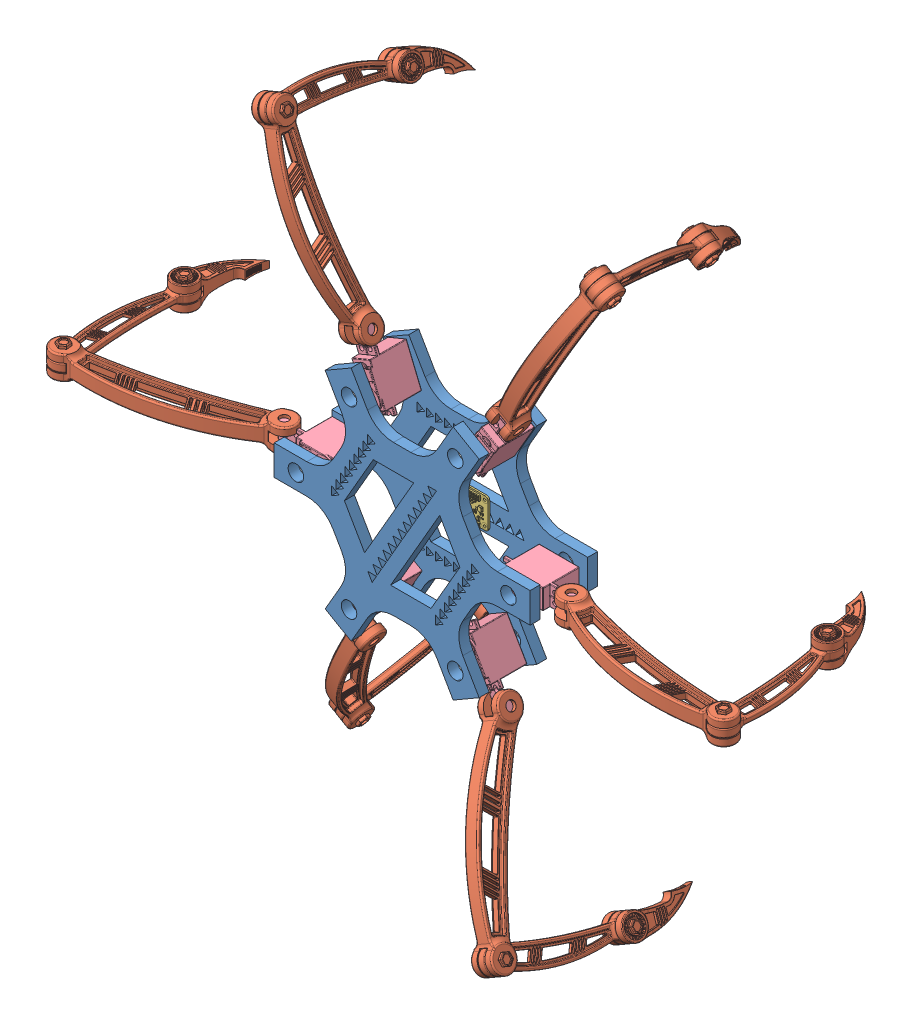
SolidWorks assembly Assem1, configuration Default. Lengths in mm.
Overall size (765.99 687.61 337.11).
15 component instances, 4 part files, 29 mates.
Components (placement in the parent):
- Upper and lower frame-1: Upper and lower frame [Default] at origin size (255.88 236.6 10)
- Leg assembly-1: Leg assembly [Default] at (-114.6549 236.1046 31.5495) x (-0.922801 -0.385273 0.001546) z (-0.324081 0.774053 -0.543887) size (30.14 189.7 217.01)
- Leg assembly-2: Leg assembly [Default] at (133.9103 223.098 16.7648) x (-0.868076 0.496428 0.002087) z (0.377645 0.663085 -0.646299) size (30.14 189.7 217.01)
- Leg assembly-4: Leg assembly [Default] at (256.5325 -7.2775 36.3251) x (-0.004411 0.999989 0.001367) z (0.860704 0.004492 -0.509086) size (30.14 189.7 217.01)
- Leg assembly-5: Leg assembly [Default] at (-117.632 -216.91 -24.8184) x (0.867543 -0.497351 0.003464) z (-0.230832 -0.408797 -0.88295) size (30.14 189.7 217.01)
- Leg assembly-6: Leg assembly [Default] at (124.234 -225.2397 76.4628) x (0.86371 0.503989 -0.000229) z (0.495439 -0.849141 -0.183032) size (30.14 189.7 217.01)
- Upper and lower frame-2: Upper and lower frame [Default] at (0 0 67.6) x (-0.5 -0.866025 0) z (0 0 -1) size (255.88 236.6 10)
- Raspberry PI Zero W-1: Raspberry PI Zero W [Default] at (-34.9564 -11.5173 10) size (65 30.65 11.38)
- Servo MG996R-1: Servo MG996R [Predeterminado] at (-87.6423 9.2686 9.4) x (-1 0 0) z (0 1 0) size (71.49 47.6 20)
- Servo MG996R-2: Servo MG996R [Predeterminado] at (55.1535 66.3846 10) x (0.5 0.866025 0) z (0.866025 -0.5 0) size (71.49 47.6 20)
- Servo MG996R-3: Servo MG996R [Predeterminado] at (30.1459 -82.5769 10) x (0.5 -0.866025 0) z (-0.866025 -0.5 0) size (71.49 47.6 20)
- Servo MG996R-4: Servo MG996R [Predeterminado] at (79.4787 -17.4288 10) x (1 0 0) z (0 -1 0) size (71.49 47.6 20)
- Servo MG996R-5: Servo MG996R [Predeterminado] at (-37.8332 76.4526 10) x (-0.381255 0.92447 0) z (0.92447 0.381255 0) size (71.49 47.6 20)
- Servo MG996R-6: Servo MG996R [Predeterminado] at (-54.8097 -69.5562 9.4) x (-0.5 -0.866025 0) z (-0.866025 0.5 0) size (71.49 47.6 20)
- Leg assembly-7: Leg assembly [Default] at (-264.095 -0.8827 49.4953) x (0.004541 -0.999989 0.000837) z (-0.91471 -0.004492 -0.404085) size (30.14 189.7 217.01)
Mates (geometry in assembly coordinates):
- Coincident2: coincident anti-aligned: plane of Leg assembly-1 through (-65.8659 130.1579 38.1282) normal (-0.92447 -0.381255 0); plane of Servo MG996R-5 through (-60.7622 117.7824 39.6) normal (0.92447 0.381255 0)
- Concentric2: concentric anti-aligned: cylinder of Leg assembly-1 through (-58.5854 133.1604 38.1282) axis (-0.92447 -0.381255 0) radius 4.5; cylinder of Servo MG996R-5 through (-77.884 125.2016 38.1282) axis (0.92447 0.381255 0) radius 4.5
- Coincident3: coincident anti-aligned: plane of Upper and lower frame-1 through (0 0 10) normal (0 0 1); plane of Servo MG996R-5 through (-56.3226 68.8275 10) normal (0 0 -1)
- Coincident4: coincident anti-aligned: plane of Upper and lower frame-1 through (0 0 10) normal (0 0 1); plane of Servo MG996R-5 through (-56.3226 68.8275 10) normal (0 0 -1)
- Coincident5: coincident anti-aligned: plane of Upper and lower frame-1 through (0 0 10) normal (0 0 1); plane of Servo MG996R-4 through (79.4787 2.5712 10) normal (0 0 -1)
- Coincident17: coincident anti-aligned: plane of Upper and lower frame-1 through (0 0 10) normal (0 0 1); plane of Servo MG996R-2 through (37.833 76.3846 10) normal (0 0 -1)
- Parallel5: parallel anti-aligned: line of Upper and lower frame-1 through (50.9808 118.3013 10) axis (0.866025 -0.5 0); line of Servo MG996R-2 through (74.7839 101.5854 10.6) axis (-0.866025 0.5 0)
- Coincident19: coincident anti-aligned: plane of Upper and lower frame-1 through (0 0 10) normal (0 0 1); plane of Servo MG996R-3 through (47.4664 -72.5769 10) normal (0 0 -1)
- Parallel6: parallel anti-aligned: line of Upper and lower frame-1 through (76.9615 -103.3013 10) axis (-0.866025 -0.5 0); line of Servo MG996R-3 through (50.8155 -117.1777 10.6) axis (0.866025 0.5 0)
- Angle3: planar angle = 0 rad anti-aligned: plane of Upper and lower frame-1 through (0 0 10) normal (0 0 1); plane of Servo MG996R-6 through (-37.4892 -79.5562 9.4) normal (0 0 -1)
- Coincident26: coincident aligned: line of Upper and lower frame-1 through (-76.9615 -103.3013 10) axis (0.866025 -0.5 0); line of Servo MG996R-6 through (-74.4401 -104.757 10) axis (0.866025 -0.5 0)
- Coincident29: coincident aligned: plane of Upper and lower frame-1; plane of Servo MG996R-1
- Parallel10: parallel anti-aligned: plane of Upper and lower frame-1 through (0 0 10) normal (0 0 1); plane of Servo MG996R-1 through (-87.6423 -10.7314 9.4) normal (0 0 -1)
- Coincident33: coincident anti-aligned: plane of Upper and lower frame-2 through (0 0 57.6) normal (0 0 -1); plane of Servo MG996R-3 through (43.8061 -86.2371 57.6) normal (0 0 1)
- Coincident36: coincident anti-aligned: plane of Leg assembly-2 through (72.7125 125.9176 38.1282) normal (0.866025 -0.5 0); plane of Servo MG996R-2 through (66.0192 114.3245 39.6) normal (-0.866025 0.5 0)
- Concentric6: concentric anti-aligned: cylinder of Leg assembly-2 through (87.4309 117.42 38.1282) axis (-0.866025 0.5 0) radius 4.5; cylinder of Servo MG996R-2 through (69.3523 127.8576 38.1282) axis (0.866025 -0.5 0) radius 4.5
- Coincident37: coincident anti-aligned: plane of Leg assembly-4 through (139.8153 -11.9888 38.1282) normal (0 1 0); plane of Servo MG996R-4 through (126.4287 -11.9888 39.6) normal (0 -1 0)
- Coincident38: coincident anti-aligned: plane of Upper and lower frame-1 through (0 0 10) normal (0 0 1); plane of Servo MG996R-4 through (79.4787 2.5712 10) normal (0 0 -1)
- Concentric7: concentric anti-aligned: cylinder of Leg assembly-4 through (139.8153 -19.8641 38.1282) axis (0 1 0) radius 4.5; cylinder of Servo MG996R-4 through (139.8153 1.0112 38.1282) axis (0 -1 0) radius 4.5
- Coincident40: coincident anti-aligned: plane of Leg assembly-6 through (72.9235 -127.5499 38.1282) normal (-0.866025 -0.5 0); plane of Servo MG996R-3 through (66.2302 -115.9568 39.6) normal (0.866025 0.5 0)
- Concentric8: concentric anti-aligned: cylinder of Leg assembly-6 through (58.2051 -136.0476 38.1282) axis (0.866025 0.5 0) radius 4.5; cylinder of Servo MG996R-3 through (76.2837 -125.6099 38.1282) axis (-0.866025 -0.5 0) radius 4.5
- Coincident41: coincident anti-aligned: plane of Upper and lower frame-1 through (0 0 10) normal (0 0 1); plane of Servo MG996R-3 through (47.4664 -72.5769 10) normal (0 0 -1)
- Coincident42: coincident aligned: plane of Leg assembly-5 through (-72.3687 -129.0892 37.5282) normal (0.866025 -0.5 0); plane of Servo MG996R-6 through (-65.6754 -117.4961 39) normal (0.866025 -0.5 0)
- Concentric10: concentric anti-aligned: cylinder of Leg assembly-5 through (-79.1889 -125.1515 37.5282) axis (0.866025 -0.5 0) radius 4.5; cylinder of Servo MG996R-6 through (-69.0085 -131.0292 37.5282) axis (-0.866025 0.5 0) radius 4.5
- Coincident43: coincident anti-aligned: plane of Servo MG996R-1 through (-134.5923 3.8286 39) normal (0 1 0); plane of Leg assembly-7 through (-147.9789 3.8286 37.5282) normal (0 -1 0)
- Coincident44: coincident anti-aligned: plane of Servo MG996R-1 through (-134.5923 -5.2914 39) normal (0 -1 0); plane of Leg assembly-7 through (-147.9789 -5.2914 37.5282) normal (0 1 0)
- Concentric12: concentric anti-aligned: cylinder of Servo MG996R-1 through (-147.9789 -9.1714 37.5282) axis (0 1 0) radius 4.5; cylinder of Leg assembly-7 through (-147.9789 11.7039 37.5282) axis (0 -1 0) radius 4.5
- Coincident45: coincident aligned: plane of Upper and lower frame-1 through (-63.9711 -110.8013 10) normal (-0.5 -0.866025 0); plane of Upper and lower frame-2 through (-63.9711 -110.8013 57.6) normal (-0.5 -0.866025 0)
- Coincident46: coincident aligned: plane of Upper and lower frame-1 through (-127.9423 0 10) normal (-1 0 0); plane of Upper and lower frame-2 through (-127.9423 0 57.6) normal (-1 0 0)
